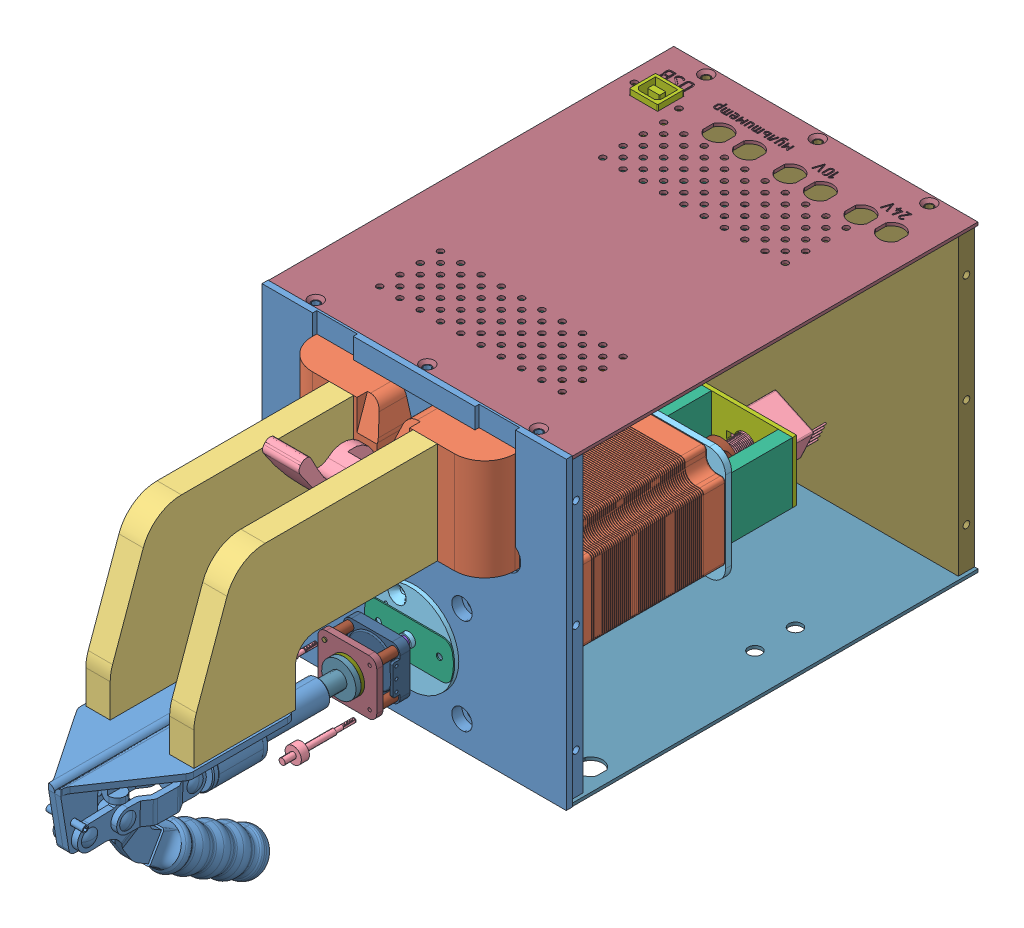
SolidWorks assembly Сборка лнейность, configuration По умолчанию. Lengths in mm.
Overall size (150 180.34 380.2).
57 component instances, 46 part files, 135 mates.
Components (placement in the parent):
- стол-1: стол [По умолчанию] at origin size (150 150 10)
- Nema 23-1: Nema 23 [По умолчанию] at (75 37 -115.5) x (0 -1 0) z (-1 0 0) size (56.72 113.5 73.51)
- подшипник-1: подшипник [По умолчанию] at (75 37 2) x (0.986309 0.164906 0) z (0 0 1) size (26 26 8)
- энкодер-1: энкодер [По умолчанию] at (63.0368 33.7853 -173.6) x (0.90717 -0.420764 0) z (0 0 1) size (21.2 15.9 49.6)
- крышка верхняя-1: крышка верхняя [По умолчанию] at (75 37 8) x (0.789196 -0.614141 0) z (0 0 1) size (44 44 6.7)
- изолятор-1: изолятор [По умолчанию] at (75 37 12) x (0.999997 -0.002629 0) z (0 0 1) size (44 19 0.6)
- ось корпус-1: ось корпус [По умолчанию] at (75 37 2) x (0.996574 0.082709 0) z (0 0 1) size (17.99 18 33.7)
- ось-1: ось [По умолчанию] at (75 37 9.6209) x (0.996574 0.082709 0) z (0 0 1) size (6.5 6.5 30.4)
- стопор оси-1: стопор оси [По умолчанию] at (75.3391 32.914 6.6209) x (-0.98067 -0.081389 0.177938) z (-0.082709 0.996574 0) size (2 2 8.5)
- стойка-1: стойка [По умолчанию] at (55.43 9 -38) x (0 1 0) z (0 0 1) size (56 8 38)
- стойка-2: стойка [По умолчанию] at (102.57 9 -38) x (0 1 0) z (0 0 1) size (56 8 38)
- муфта-1: муфта [По умолчанию] at (75 37 -121.5) x (-0.99255 0.121836 0) z (0 0 -1) size (17.99 18 20)
- основание-1: основание [По умолчанию] at (1.7 1.7 -193) size (146.6 146.6 8)
- стенка бок-1: стенка бок [По умолчанию] at (149.8 148.3 -193) x (0 -1 0) z (-1 0 0) size (146.6 200 1.5) (hidden)
- стенка зад-1: стенка зад [По умолчанию] at (0 149.8 -193) x (1 0 0) z (0 -1 0) size (150 200 1.5)
- стенка перед-1: стенка перед [По умолчанию] at (150 0.2 -193) x (-1 0 0) z (0 1 0) size (150 200 1.5)
- драйвер-1: драйвер [По умолчанию] at (1.7 126.8 -145) x (1 0 0) z (0 -1 0) size (75 118 32)
- стенка бок 2-1: стенка бок 2 [По умолчанию] at (0.2 1.7 -193) x (0 1 0) z (1 0 0) size (146.6 200 1.5)
- стойка для платы-1: стойка для платы [По умолчанию] at (9.7 26.7 -148) x (0 0 1) z (-1 0 0) size (8 8 8)
- стойка для платы-2: стойка для платы [По умолчанию] at (9.7 80.7 -148) x (0 0 1) z (-1 0 0) size (8 8 8)
- стойка для платы-3: стойка для платы [По умолчанию] at (9.7 80.7 -64) x (0 0 1) z (-1 0 0) size (8 8 8)
- стойка для платы-4: стойка для платы [По умолчанию] at (9.7 26.7 -64) x (0 0 1) z (-1 0 0) size (8 8 8)
- плата-1: плата [По умолчанию] at (9.7 18.7 -156) x (0 1 0) z (1 0 0) size (70 100 9)
- прижим-1: прижим [По умолчанию] at (75.5899 43.7042 131.1718) x (0 0 1) z (0 -1 0) size (129.93 55.6 84)
- стойка прижима основа-1: стойка прижима основа [По умолчанию] at (25 140 8) x (0 -1 0) z (0 0 1) size (50 100 17.2)
- стойка прижима держатель-1: стойка прижима держатель [По умолчанию] at (48.35 61.4042 95.2) x (0 1 0) z (1 0 0) size (78.62 120 12)
- стойка прижима держатель-2: стойка прижима держатель [По умолчанию] at (89.65 61.4042 95.2) x (0 1 0) z (1 0 0) size (78.62 120 12)
- плата для замеров-1: плата для замеров [По умолчанию] at (75 37 10) size (150 90 3) (hidden)
- винт-1: винт [По умолчанию] at (86.8379 27.7879 51.4405) x (0.711974 0.702205 0) z (0 0 1) size (8 8 35.5)
- винт-2: винт [По умолчанию] at (63.1621 46.2121 46.6645) x (-0.879742 0.475451 0) z (0 0 1) size (8 8 35.5)
- держатель энкодера пластина-1: держатель энкодера пластина [По умолчанию] at (47 65 -118.5) x (0 -1 0) z (0 0 1) size (56 56 3)
- держатель энкодера стойка-1: держатель энкодера стойка [По умолчанию] at (51.5 52 -118.5) x (0 -1 0) z (1 0 0) size (30 34.6 7)
- держатель энкодера стойка-2: держатель энкодера стойка [По умолчанию] at (91.5 52 -118.5) x (0 -1 0) z (1 0 0) size (30 34.6 7)
- держатель энкодера крышка-1: держатель энкодера крышка [По умолчанию] at (98.5 22 -153.1) x (-1 0 0) z (0 0 -1) size (47 30 2)
- гайка-1: гайка [По умолчанию] at (75 115 -1.7) x (-1 0 0) z (0 0 1) size (13 13 5.9)
- фиксатор-1: фиксатор [По умолчанию] at (60 107.5 -3.2) size (30 15 3)
- п_крышка.stp-2: п_крышка.stp [По умолчанию] at (75 37.0042 34.5225) x (-1 0 0) z (0 0 -1) size (28 26 8.5)
- стойка крышка-1: стойка крышка [По умолчанию] at (86 27.5042 30.9225) size (4.4 4.4 9)
- стойка крышка-2: стойка крышка [По умолчанию] at (64 46.5042 30.9225) size (4.4 4.4 9)
- стойка крышка-3: стойка крышка [По умолчанию] at (64 27.5042 30.9225) size (4.4 4.4 9)
- стойка крышка-4: стойка крышка [По умолчанию] at (86 46.5042 30.9225) size (4.4 4.4 9)
- винт 2-1: винт 2 [По умолчанию] at (64 46.5042 26.1225) size (3.7 3.7 17.3)
- прижим крышки-1: прижим крышки [По умолчанию] at (60.5 23.5042 39.9225) size (29 27 3)
- винт опора крышки-1: винт опора крышки [По умолчанию] at (75 37.0042 47.1225) x (-0.478283 -0.878206 0) z (0 0 -1) size (17 17 37.2)
- шайба прижима-1: шайба прижима [По умолчанию] at (75 37.0042 39.9225) x (-0.50555 -0.862797 0) z (0 0 -1) size (17 17 2)
- резина-1: резина [По умолчанию] at (75 37.0042 42.9225) size (17 17 1.7)
- п_корпус.stp-1: п_корпус.stp [По умолчанию] at (75 37 25.1) x (0.051325 0.998682 0) z (0 0 -1) size (28 36 12.5) (hidden)
- держатель датчика-1: держатель датчика [По умолчанию] at (48.57 66.5 -36.15) x (1 0 0) z (0 -1 0) size (55 25 1.5)
- датчик-1: датчик [По умолчанию] at (81.195 58.34 -3.05) x (0 0 -1) z (0 1 0) size (33.3 10.25 18.74)
- диск датчика-1: диск датчика [По умолчанию] at (75 37 -25) x (-0.996574 -0.082709 0) z (0 0 1) size (37 37 1.5)
- датчик стойка-1: датчик стойка [По умолчанию] at (76.07 60 -33.15) x (1 0 0) z (0 1 0) size (6 6 5)
- датчик стойка-2: датчик стойка [По умолчанию] at (76.07 60 -14.15) x (1 0 0) z (0 1 0) size (6 6 5)
- контакт-1: контакт [По умолчанию] at (75 37.0042 29.5225) size (21.8 21.8 0.8)
- эксцентрик-1: эксцентрик [По умолчанию] at (65.95 117.2509 36.0167) x (0 0.661095 0.750303) z (1 0 0) size (59.77 22.47 18)
- штифт эксцентрика-1: штифт эксцентрика [По умолчанию] at (83.95 115 38) x (0 0.994131 -0.108185) z (-1 0 0) size (6 6 18)
- винт эксцентрика-1: винт эксцентрика [По умолчанию] at (75 115 -23) x (0 1 0) z (0 0 1) size (14 8 68)
- разъем USB-1: разъем USB [По умолчанию] at (7.8 148.3 -176.75) x (1 0 0) z (0 -1 0) size (28 18 18.8)
Mates (geometry in assembly coordinates):
- Параллельность1: parallel anti-aligned: plane of стол-1 through (0 0 0) normal (0 0 -1); plane of Nema 23-1 through (75 37 -36.5) normal (0 0 1)
- Параллельность2: parallel aligned: plane of стол-1 through (0 0 10) normal (0 -1 0); plane of Nema 23-1 through (58 8.85 -38) normal (0 -1 0)
- Концентричный15: concentric anti-aligned: cylinder of Nema 23-1 through (75 37 -130.5) axis (0 0 1) radius 4; cylinder of энкодер-1 through (75 37 -132.5) axis (0 0 -1) radius 3.15
- Совпадение18: coincident anti-aligned: plane of стол-1 through (75 37 2) normal (0 0 1); plane of подшипник-1 through (75 37 2) normal (0 0 -1)
- Концентричный16: concentric anti-aligned: cylinder of стол-1 through (75 37 2) axis (0 0 1) radius 13; cylinder of подшипник-1 through (75 37 10) axis (0 0 -1) radius 13
- Совпадение19: coincident anti-aligned: plane of стол-1 through (75 37 8) normal (0 0 1); plane of крышка верхняя-1 through (75 37 8) normal (0 0 -1)
- Совпадение20: coincident anti-aligned: plane of крышка верхняя-1 through (75 37 12) normal (0 0 1); plane of изолятор-1 through (75 37 12) normal (0 0 -1)
- Концентричный20: concentric anti-aligned: cylinder of крышка верхняя-1 through (75 37 14.7) axis (0 0 -1) radius 3.25; cylinder of изолятор-1 through (75 37 12) axis (0 0 1) radius 3.25
- Концентричный21: concentric anti-aligned: cylinder of подшипник-1 through (75 37 10) axis (0 0 -1) radius 4.5; cylinder of крышка верхняя-1 through (75 37 8) axis (0 0 1) radius 2.5
- Концентричный23: concentric aligned: cylinder of подшипник-1 through (75 37 10) axis (0 0 -1) radius 4.5; cylinder of ось корпус-1 through (75 37 9.7) axis (0 0 -1) radius 4.5
- Концентричный24: concentric anti-aligned: cylinder of ось-1 through (75.2688 33.7611 6.6209) axis (-0.082709 0.996574 0) radius 1; cylinder of стопор оси-1 through (74.6361 41.3849 6.6209) axis (0.082709 -0.996574 0) radius 1
- Расстояние3: distance = 4.1 mm: cylinder of ось-1 through (75 37 -5.3791) axis (0 0 1) radius 3.25; plane of стопор оси-1 through (75.3391 32.914 6.6209) normal (0.082709 -0.996574 0)
- Концентричный25: concentric aligned: cylinder of ось корпус-1 through (75 37 -16.3) axis (0 0 1) radius 3.25; cylinder of ось-1 through (75 37 -5.3791) axis (0 0 1) radius 3.25
- Параллельность3: parallel anti-aligned: cylinder of ось корпус-1 through (75.579 30.024 3) axis (-0.082709 0.996574 0) radius 1; cylinder of стопор оси-1 through (74.6361 41.3849 6.6209) axis (0.082709 -0.996574 0) radius 1
- Совпадение24: coincident anti-aligned: plane of подшипник-1 through (75 37 2) normal (0 0 -1); plane of ось корпус-1 through (75 37 2) normal (0 0 1)
- Совпадение32: coincident anti-aligned: plane of стол-1 through (0 0 0) normal (0 0 -1); plane of стойка-2 through (102.57 9 0) normal (0 0 1)
- Совпадение33: coincident anti-aligned: plane of стол-1 through (0 0 0) normal (0 0 -1); plane of стойка-1 through (55.43 9 0) normal (0 0 1)
- Концентричный29: concentric aligned: cylinder of стол-1 through (98.57 60.57 0) axis (0 0 1) radius 2.5; cylinder of стойка-2 through (98.57 60.57 -38) axis (0 0 1) radius 2.1
- Концентричный30: concentric aligned: cylinder of стол-1 through (98.57 13.43 0) axis (0 0 1) radius 2.5; cylinder of стойка-2 through (98.57 13.43 -38) axis (0 0 1) radius 2.1
- Концентричный31: concentric aligned: cylinder of стол-1 through (51.43 60.57 0) axis (0 0 1) radius 2.5; cylinder of стойка-1 through (51.43 60.57 -38) axis (0 0 1) radius 2.1
- Концентричный32: concentric aligned: cylinder of стол-1 through (51.43 13.43 0) axis (0 0 1) radius 2.5; cylinder of стойка-1 through (51.43 13.43 -38) axis (0 0 1) radius 2.1
- Совпадение34: coincident anti-aligned: plane of Nema 23-1 through (101.15 20 -38) normal (0 0 1); plane of стойка-1 through (55.43 9 -38) normal (0 0 -1)
- Концентричный33: concentric aligned: cylinder of Nema 23-1 through (75 37 -17) axis (0 0 -1) radius 4; cylinder of ось корпус-1 through (75 37 -16) axis (0 0 -1) radius 4
- Концентричный35: concentric aligned: cylinder of Nema 23-1 through (75 37 -130.5) axis (0 0 1) radius 4; cylinder of муфта-1 through (75 37 -131.5) axis (0 0 1) radius 4
- Расстояние4: distance = 1 mm anti-aligned: plane of Nema 23-1 through (75 37 -130.5) normal (0 0 -1); plane of муфта-1 through (75 37 -131.5) normal (0 0 1)
- Расстояние5: distance = 1 mm aligned: plane of энкодер-1 through (75 37 -132.5) normal (0 0 1); plane of муфта-1 through (75 37 -131.5) normal (0 0 1)
- Совпадение40: coincident anti-aligned: plane of основание-1 through (148.3 1.7 -185) normal (1 0 0); plane of стенка бок-1 through (148.3 148.3 -193) normal (-1 0 0)
- Концентричный40: concentric aligned: cylinder of основание-1 through (148.3 128.3 -189) axis (-1 0 0) radius 1.65; cylinder of стенка бок-1 through (149.8 128.3 -189) axis (-1 0 0) radius 2
- Концентричный41: concentric aligned: cylinder of основание-1 through (148.3 21.7 -189) axis (-1 0 0) radius 1.65; cylinder of стенка бок-1 through (149.8 21.7 -189) axis (-1 0 0) radius 2
- Совпадение41: coincident anti-aligned: plane of основание-1 through (1.7 148.3 -185) normal (0 1 0); plane of стенка зад-1 through (0 148.3 -193) normal (0 -1 0)
- Концентричный42: concentric aligned: cylinder of основание-1 through (130 148.3 -189) axis (0 -1 0) radius 1.65; cylinder of стенка зад-1 through (130 149.8 -189) axis (0 -1 0) radius 2
- Концентричный43: concentric anti-aligned: cylinder of стол-1 through (20 133.3 3.5) axis (0 1 0) radius 1.65; cylinder of стенка зад-1 through (20 149.8 3.5) axis (0 -1 0) radius 2
- Совпадение42: coincident anti-aligned: plane of стол-1 through (148.3 1.7 7) normal (0 -1 0); plane of стенка перед-1 through (150 1.7 -193) normal (0 1 0)
- Концентричный45: concentric anti-aligned: cylinder of основание-1 through (20 148.3 -189) axis (0 -1 0) radius 1.65; cylinder of стенка перед-1 through (20 0.2 -189) axis (0 1 0) radius 2
- Концентричный46: concentric anti-aligned: cylinder of основание-1 through (130 148.3 -189) axis (0 -1 0) radius 1.65; cylinder of стенка перед-1 through (130 0.2 -189) axis (0 1 0) radius 2
- Совпадение45: coincident anti-aligned: plane of стол-1 through (1.7 148.3 7) normal (-1 0 0); plane of стенка бок 2-1 through (1.7 1.7 -193) normal (1 0 0)
- Концентричный48: concentric anti-aligned: cylinder of стол-1 through (16.7 21.7 3.5) axis (-1 0 0) radius 1.65; cylinder of стенка бок 2-1 through (0.2 21.7 3.5) axis (1 0 0) radius 2
- Концентричный49: concentric anti-aligned: cylinder of стол-1 through (16.7 128.3 3.5) axis (-1 0 0) radius 1.65; cylinder of стенка бок 2-1 through (0.2 128.3 3.5) axis (1 0 0) radius 2
- Параллельность5: parallel anti-aligned: plane of стенка зад-1 through (0 148.3 -193) normal (0 -1 0); plane of драйвер-1 through (1.7 140.8 -145) normal (0 1 0)
- Совпадение48: coincident anti-aligned: plane of стол-1 through (148.3 148.3 7) normal (1 0 0); plane of стенка бок-1 through (148.3 148.3 -193) normal (-1 0 0)
- Концентричный51: concentric anti-aligned: cylinder of стол-1 through (133.3 21.7 3.5) axis (1 0 0) radius 1.65; cylinder of стенка бок-1 through (149.8 21.7 3.5) axis (-1 0 0) radius 2
- Совпадение49: coincident anti-aligned: plane of стенка бок 2-1 through (1.7 1.7 -193) normal (1 0 0); plane of стойка для платы-4 through (1.7 26.7 -64) normal (-1 0 0)
- Совпадение50: coincident anti-aligned: plane of стенка бок 2-1 through (1.7 1.7 -193) normal (1 0 0); plane of стойка для платы-2 through (1.7 80.7 -148) normal (-1 0 0)
- Совпадение51: coincident anti-aligned: plane of стенка бок 2-1 through (1.7 1.7 -193) normal (1 0 0); plane of стойка для платы-3 through (1.7 80.7 -64) normal (-1 0 0)
- Совпадение52: coincident anti-aligned: plane of стенка бок 2-1 through (1.7 1.7 -193) normal (1 0 0); plane of стойка для платы-1 through (1.7 26.7 -148) normal (-1 0 0)
- Совпадение53: coincident anti-aligned: plane of стойка для платы-3 through (9.7 80.7 -64) normal (1 0 0); plane of плата-1 through (9.7 18.7 -156) normal (-1 0 0)
- Концентричный52: concentric aligned: cylinder of стойка для платы-3 through (1.7 80.7 -64) axis (1 0 0) radius 2; cylinder of плата-1 through (9.7 80.7 -64) axis (1 0 0) radius 2
- Концентричный53: concentric aligned: cylinder of стойка для платы-2 through (1.7 80.7 -148) axis (1 0 0) radius 2; cylinder of плата-1 through (9.7 80.7 -148) axis (1 0 0) radius 2
- Концентричный54: concentric aligned: cylinder of стойка для платы-1 through (1.7 26.7 -148) axis (1 0 0) radius 2; cylinder of плата-1 through (9.7 26.7 -148) axis (1 0 0) radius 2
- Концентричный55: concentric aligned: cylinder of стойка для платы-4 through (1.7 26.7 -64) axis (1 0 0) radius 2; cylinder of плата-1 through (9.7 26.7 -64) axis (1 0 0) radius 2
- Концентричный56: concentric aligned: cylinder of стенка бок 2-1 through (0.2 80.7 -64) axis (1 0 0) radius 2; cylinder of стойка для платы-3 through (1.7 80.7 -64) axis (1 0 0) radius 2
- Концентричный57: concentric aligned: cylinder of стенка бок 2-1 through (0.2 26.7 -64) axis (1 0 0) radius 2; cylinder of стойка для платы-4 through (1.7 26.7 -64) axis (1 0 0) radius 2
- Совпадение74: coincident anti-aligned: plane of драйвер-1 through (1.7 108.8 -145) normal (-1 0 0); plane of стенка бок 2-1 through (1.7 1.7 -193) normal (1 0 0)
- Концентричный61: concentric anti-aligned: cylinder of драйвер-1 through (76.7 118.3 -148) axis (-1 0 0) radius 2.5; cylinder of стенка бок 2-1 through (0.2 118.3 -148) axis (1 0 0) radius 2
- Концентричный69: concentric aligned: cylinder of стол-1 through (75 115 0) axis (0 0 1) radius 3; cylinder of стойка прижима основа-1 through (75 115 8) axis (0 0 1) radius 3
- Совпадение81: coincident anti-aligned: plane of стол-1 through (25 90 8) normal (0 1 0); plane of стойка прижима основа-1 through (25 90 25.2) normal (0 -1 0)
- Совпадение82: coincident anti-aligned: plane of стойка прижима основа-1 through (25 140 25.2) normal (0 0 1); plane of стойка прижима держатель-1 through (-46.0026 90 25.2) normal (0 0 -1)
- Совпадение83: coincident anti-aligned: plane of стойка прижима основа-1 through (25 140 25.2) normal (0 0 1); plane of стойка прижима держатель-2 through (-4.7026 90 25.2) normal (0 0 -1)
- Концентричный70: concentric aligned: cylinder of стойка прижима основа-1 through (95.65 100 25.2) axis (0 0 -1) radius 3; cylinder of стойка прижима держатель-2 through (95.65 100 55.2) axis (0 0 -1) radius 2.5
- Параллельность10: parallel aligned: plane of стол-1 through (0 150 10) normal (0 1 0); plane of прижим-1 through (52.2 61.4042 146.67) normal (0 1 0)
- Концентричный78: concentric aligned: cylinder of стойка прижима основа-1 through (54.35 130 25.2) axis (0 0 -1) radius 3; cylinder of стойка прижима держатель-1 through (54.35 130 55.2) axis (0 0 -1) radius 2.5
- Концентричный79: concentric aligned: cylinder of прижим-1 through (95.65 63.1042 136.2) axis (0 -1 0) radius 2.6; cylinder of стойка прижима держатель-2 through (95.65 81.4042 136.2) axis (0 -1 0) radius 2.5
- Совпадение87: coincident anti-aligned: plane of прижим-1 through (97.8 61.4042 146.67) normal (0 1 0); plane of стойка прижима держатель-2 through (101.65 61.4042 95.2) normal (0 -1 0)
- Концентричный80: concentric aligned: cylinder of крышка верхняя-1 through (75 37 12) axis (0 0 -1) radius 22; cylinder of плата для замеров-1 through (75 37 13) axis (0 0 -1) radius 22
- Концентричный81: concentric anti-aligned: cylinder of крышка верхняя-1 through (86.8379 27.7879 8) axis (0 0 1) radius 0.8; cylinder of винт-1 through (86.8379 27.7879 61.4405) axis (0 0 -1) radius 1
- Концентричный82: concentric anti-aligned: cylinder of крышка верхняя-1 through (63.1621 46.2121 8) axis (0 0 1) radius 0.8; cylinder of винт-2 through (63.1621 46.2121 56.6645) axis (0 0 -1) radius 1
- Совпадение92: coincident anti-aligned: plane of Nema 23-1 through (75 37 -115.5) normal (0 0 -1); plane of держатель энкодера пластина-1 through (95 17 -115.5) normal (0 0 1)
- Концентричный84: concentric anti-aligned: cylinder of Nema 23-1 through (59 11.67 -111.5) axis (0 0 -1) radius 1.25; cylinder of держатель энкодера пластина-1 through (59 11.67 -118.5) axis (0 0 1) radius 1.5
- Концентричный85: concentric anti-aligned: cylinder of Nema 23-1 through (91 62.33 -111.5) axis (0 0 -1) radius 1.25; cylinder of держатель энкодера пластина-1 through (91 62.33 -118.5) axis (0 0 1) radius 1.5
- Совпадение93: coincident anti-aligned: plane of держатель энкодера пластина-1 through (95 17 -118.5) normal (0 0 -1); plane of держатель энкодера стойка-1 through (58.5 52 -118.5) normal (0 0 1)
- Совпадение94: coincident anti-aligned: plane of держатель энкодера пластина-1 through (95 17 -118.5) normal (0 0 -1); plane of держатель энкодера стойка-2 through (98.5 52 -118.5) normal (0 0 1)
- Совпадение95: coincident anti-aligned: plane of держатель энкодера стойка-1 through (58.5 52 -153.1) normal (0 0 -1); plane of держатель энкодера крышка-1 through (98.5 22 -153.1) normal (0 0 1)
- Концентричный94: concentric aligned: cylinder of держатель энкодера стойка-2 through (95 48 -118.5) axis (0 0 -1) radius 1.25; cylinder of держатель энкодера крышка-1 through (95 48 -153.1) axis (0 0 -1) radius 1.5
- Концентричный95: concentric anti-aligned: cylinder of держатель энкодера пластина-1 through (55 26 -118.5) axis (0 0 1) radius 1.5; cylinder of держатель энкодера стойка-1 through (55 26 -118.5) axis (0 0 -1) radius 1.25
- Концентричный97: concentric anti-aligned: cylinder of держатель энкодера пластина-1 through (55 48 -118.5) axis (0 0 1) radius 1.5; cylinder of держатель энкодера стойка-1 through (55 48 -118.5) axis (0 0 -1) radius 1.25
- Концентричный98: concentric anti-aligned: cylinder of держатель энкодера пластина-1 through (95 26 -118.5) axis (0 0 1) radius 1.5; cylinder of держатель энкодера стойка-2 through (95 26 -118.5) axis (0 0 -1) radius 1.25
- Концентричный99: concentric anti-aligned: cylinder of держатель энкодера пластина-1 through (95 48 -118.5) axis (0 0 1) radius 1.5; cylinder of держатель энкодера стойка-2 through (95 48 -118.5) axis (0 0 -1) radius 1.25
- Концентричный100: concentric aligned: cylinder of держатель энкодера стойка-1 through (55 26 -118.5) axis (0 0 -1) radius 1.25; cylinder of держатель энкодера крышка-1 through (55 26 -153.1) axis (0 0 -1) radius 1.5
- Совпадение96: coincident anti-aligned: plane of стол-1 through (0 0 0) normal (0 0 -1); plane of гайка-1 through (75 115 0) normal (0 0 1)
- Совпадение97: coincident anti-aligned: plane of стол-1 through (69.2265 115 4) normal (0.866025 -0.5 0); plane of гайка-1 through (72.1132 120 25.3753) normal (-0.866025 0.5 0)
- Концентричный102: concentric aligned: cylinder of стол-1 through (75 115 0) axis (0 0 1) radius 3; cylinder of гайка-1 through (75 115 -1.7) axis (0 0 1) radius 2.5
- Совпадение98: coincident aligned: circle of гайка-1; plane of фиксатор-1 through (75 115 -1.7) normal (0 0 1)
- Концентричный103: concentric aligned: cylinder of стол-1 through (75 115 0) axis (0 0 1) radius 3; cylinder of фиксатор-1 through (75 115 -3.2) axis (0 0 1) radius 3.25
- Совпадение99: coincident anti-aligned: plane of стол-1 through (0 0 10) normal (0 0 1); plane of плата для замеров-1 through (149 89 10) normal (0 0 -1)
- Параллельность12: parallel aligned: plane of стол-1 through (1.7 148.3 7) normal (-1 0 0); plane of плата для замеров-1 through (0 89 13) normal (-1 0 0)
- Совпадение100: coincident aligned: plane of стойка крышка-3 through (64 27.5042 30.9225) normal (0 0 -1); plane of стойка крышка-4 through (86 46.5042 30.9225) normal (0 0 -1)
- Совпадение101: coincident aligned: plane of стойка крышка-2 through (64 46.5042 30.9225) normal (0 0 -1); plane of стойка крышка-3 through (64 27.5042 30.9225) normal (0 0 -1)
- Совпадение102: coincident aligned: plane of стойка крышка-1 through (86 27.5042 30.9225) normal (0 0 -1); plane of стойка крышка-2 through (64 46.5042 30.9225) normal (0 0 -1)
- Совпадение103: coincident anti-aligned: plane of п_крышка.stp-2 through (75 37.0042 30.9225) normal (0 0 1); plane of стойка крышка-1 through (86 27.5042 30.9225) normal (0 0 -1)
- Концентричный104: concentric anti-aligned: cylinder of п_крышка.stp-2 through (86 27.5042 -2.0775) axis (0 0 1) radius 1.2; cylinder of стойка крышка-1 through (86 27.5042 39.9225) axis (0 0 -1) radius 1.2
- Концентричный105: concentric anti-aligned: cylinder of п_крышка.stp-2 through (86 46.5042 -2.0775) axis (0 0 1) radius 1.2; cylinder of стойка крышка-4 through (86 46.5042 39.9225) axis (0 0 -1) radius 1.2
- Концентричный106: concentric anti-aligned: cylinder of п_крышка.stp-2 through (64 46.5042 -2.0775) axis (0 0 1) radius 1.2; cylinder of стойка крышка-2 through (64 46.5042 39.9225) axis (0 0 -1) radius 1.2
- Концентричный107: concentric anti-aligned: cylinder of п_крышка.stp-2 through (64 27.5042 -2.0775) axis (0 0 1) radius 1.2; cylinder of стойка крышка-3 through (64 27.5042 39.9225) axis (0 0 -1) radius 1.2
- Концентричный108: concentric anti-aligned: cylinder of п_крышка.stp-2 through (64 46.5042 -2.0775) axis (0 0 1) radius 1.2; cylinder of винт 2-1 through (64 46.5042 63.5509) axis (0 0 -1) radius 1
- Совпадение104: coincident anti-aligned: plane of п_крышка.stp-2 through (64 46.5042 27.5225) normal (0 0 -1); plane of винт 2-1 through (64 46.5042 27.5225) normal (0 0 1)
- Совпадение105: coincident anti-aligned: plane of стойка крышка-2 through (64 46.5042 39.9225) normal (0 0 1); plane of прижим крышки-1 through (64.5 27.5042 39.9225) normal (0 0 -1)
- Концентричный109: concentric anti-aligned: cylinder of стойка крышка-4 through (86 46.5042 39.9225) axis (0 0 -1) radius 1.2; cylinder of прижим крышки-1 through (86 46.5042 39.9225) axis (0 0 1) radius 0.8
- Концентричный110: concentric anti-aligned: cylinder of стойка крышка-3 through (64 27.5042 39.9225) axis (0 0 -1) radius 1.2; cylinder of прижим крышки-1 through (64 27.5042 39.9225) axis (0 0 1) radius 0.8
- Концентричный111: concentric aligned: cylinder of прижим-1 through (75 37.0042 132.1147) axis (0 0 -1) radius 6.35; cylinder of винт опора крышки-1 through (75 37.0042 77.1225) axis (0 0 -1) radius 4
- Концентричный112: concentric aligned: cylinder of прижим крышки-1 through (75 37.0042 39.9225) axis (0 0 1) radius 4.5; cylinder of винт опора крышки-1 through (75 37.0042 39.9225) axis (0 0 1) radius 4
- Концентричный113: concentric aligned: cylinder of прижим-1 through (54.35 63.1042 102.2) axis (0 -1 0) radius 2.6; cylinder of стойка прижима держатель-1 through (54.35 81.4042 102.2) axis (0 -1 0) radius 2.5
- Концентричный114: concentric anti-aligned: cylinder of винт опора крышки-1 through (75 37.0042 39.9225) axis (0 0 1) radius 4; circle of шайба прижима-1
- Совпадение108: coincident anti-aligned: plane of винт опора крышки-1 through (75 37.0042 39.9225) normal (0 0 -1); plane of шайба прижима-1 through (75 37.0042 39.9225) normal (0 0 1)
- Совпадение109: coincident anti-aligned: plane of винт опора крышки-1 through (75 37.0042 44.6225) normal (0 0 -1); plane of резина-1 through (75 37.0042 44.6225) normal (0 0 1)
- Концентричный115: concentric anti-aligned: cylinder of винт опора крышки-1 through (75 37.0042 39.9225) axis (0 0 1) radius 4; cylinder of резина-1 through (75 37.0042 44.6225) axis (0 0 -1) radius 4
- Совпадение110: coincident anti-aligned: plane of прижим крышки-1 through (64.5 27.5042 42.9225) normal (0 0 1); plane of резина-1 through (75 37.0042 42.9225) normal (0 0 -1)
- Параллельность13: parallel aligned: plane of стойка прижима основа-1 through (25 90 25.2) normal (0 -1 0); plane of прижим крышки-1 through (64.5 23.5042 42.9225) normal (0 -1 0)
- Совпадение112: coincident anti-aligned: plane of стол-1 through (0 0 8) normal (0 0 1); plane of стойка прижима основа-1 through (25 140 8) normal (0 0 -1)
- Совпадение113: coincident anti-aligned: plane of изолятор-1 through (75 37 12.6) normal (0 0 1); plane of п_корпус.stp-1 through (75 37 12.6) normal (0 0 -1)
- Концентричный116: concentric aligned: cylinder of крышка верхняя-1 through (75 37 14.7) axis (0 0 -1) radius 3.25; cylinder of п_корпус.stp-1 through (75 37 25.1) axis (0 0 -1) radius 2.5
- Совпадение114: coincident anti-aligned: plane of стойка-2 through (102.57 65 0) normal (0 1 0); plane of держатель датчика-1 through (48.57 65 -36.15) normal (0 -1 0)
- Параллельность16: parallel aligned: plane of стойка-1 through (47.43 9 0) normal (-1 0 0); plane of держатель датчика-1 through (48.57 65 -36.15) normal (-1 0 0)
- Концентричный123: concentric anti-aligned: cylinder of Nema 23-1 through (75 37 -17) axis (0 0 -1) radius 4; cylinder of диск датчика-1 through (75 37 -25) axis (0 0 1) radius 4
- Совпадение116: coincident anti-aligned: plane of ось корпус-1 through (75 37 -24) normal (0 0 -1); plane of диск датчика-1 through (75 37 -24) normal (0 0 1)
- Параллельность17: parallel aligned: plane of ось корпус-1 through (42.1379 33.9716 -26) normal (-0.082709 0.996574 0); plane of диск датчика-1 through (72.5324 36.3437 -25) normal (-0.082709 0.996574 0)
- Совпадение118: coincident aligned: plane of датчик стойка-1 through (76.07 65 -33.15) normal (0 1 0); plane of датчик стойка-2 through (76.07 65 -14.15) normal (0 1 0)
- Совпадение119: coincident anti-aligned: plane of держатель датчика-1 through (48.57 65 -36.15) normal (0 -1 0); plane of датчик стойка-2 through (76.07 65 -14.15) normal (0 1 0)
- Концентричный124: concentric aligned: cylinder of держатель датчика-1 through (76.07 66.5 -33.15) axis (0 -1 0) radius 1.6; cylinder of датчик стойка-1 through (76.07 65 -33.15) axis (0 -1 0) radius 1.65
- Концентричный125: concentric aligned: cylinder of держатель датчика-1 through (76.07 66.5 -14.15) axis (0 -1 0) radius 1.6; cylinder of датчик стойка-2 through (76.07 65 -14.15) axis (0 -1 0) radius 1.65
- Совпадение120: coincident anti-aligned: plane of датчик-1 through (81.195 60 -3.05) normal (0 1 0); plane of датчик стойка-2 through (76.07 60 -14.15) normal (0 -1 0)
- Концентричный126: concentric anti-aligned: cylinder of датчик-1 through (76.07 58.34 -14.15) axis (0 1 0) radius 1.7; cylinder of датчик стойка-2 through (76.07 65 -14.15) axis (0 -1 0) radius 1.65
- Концентричный127: concentric anti-aligned: cylinder of датчик-1 through (76.07 58.34 -33.15) axis (0 1 0) radius 1.7; cylinder of датчик стойка-1 through (76.07 65 -33.15) axis (0 -1 0) radius 1.65
- Концентричный128: concentric anti-aligned: cylinder of стойка-2 through (98.57 45 -19) axis (0 1 0) radius 1.25; cylinder of держатель датчика-1 through (98.57 66.5 -19) axis (0 -1 0) radius 1.6
- Совпадение121: coincident anti-aligned: plane of п_крышка.stp-2 through (75 37.0042 30.3225) normal (0 0 -1); plane of контакт-1 through (75 37.0042 30.3225) normal (0 0 1)
- Концентричный129: concentric aligned: cylinder of п_крышка.stp-2 through (75 37.0042 30.2225) axis (0 0 -1) radius 3.5; cylinder of контакт-1 through (75 37.0042 30.3225) axis (0 0 -1) radius 4.9
- Концентричный130: concentric anti-aligned: cylinder of стол-1 through (75 115 0) axis (0 0 1) radius 3; cylinder of винт эксцентрика-1 through (75 115 32) axis (0 0 -1) radius 3
- Параллельность18: parallel anti-aligned: plane of стойка прижима держатель-1 through (60.35 61.4042 95.2) normal (1 0 0); plane of винт эксцентрика-1 through (71 115 38) normal (-1 0 0)
- Концентричный131: concentric anti-aligned: cylinder of эксцентрик-1 through (70.5147 115 38) axis (1 0 0) radius 3; cylinder of винт эксцентрика-1 through (79 115 38) axis (-1 0 0) radius 3
- Совпадение123: coincident anti-aligned: plane of эксцентрик-1 through (79 118.2322 20.4913) normal (-1 0 0); plane of винт эксцентрика-1 through (79 115 38) normal (1 0 0)
- Концентричный132: concentric aligned: cylinder of эксцентрик-1 through (65.95 115 38) axis (1 0 0) radius 2.1; cylinder of штифт эксцентрика-1 through (70.95 115 38) axis (1 0 0) radius 3
- Совпадение124: coincident aligned: plane of эксцентрик-1 through (83.95 117.2509 36.0167) normal (1 0 0); plane of штифт эксцентрика-1 through (83.95 115 38) normal (1 0 0)
- Расстояние6: distance = 23 mm aligned: plane of стол-1 through (0 0 0) normal (0 0 -1); plane of винт эксцентрика-1 through (75 115 -23) normal (0 0 -1)
- Совпадение125: coincident anti-aligned: plane of стенка зад-1 through (0 148.3 -193) normal (0 -1 0); plane of разъем USB-1 through (9.3 148.3 -175.25) normal (0 1 0)
- Концентричный133: concentric aligned: cylinder of стенка зад-1 through (27.8 148.3 -167.75) axis (0 1 0) radius 1.55; cylinder of разъем USB-1 through (27.8 133.8 -167.75) axis (0 1 0) radius 1.25
- Концентричный134: concentric aligned: cylinder of стенка зад-1 through (5.8 148.3 -167.75) axis (0 1 0) radius 1.55; cylinder of разъем USB-1 through (5.8 133.8 -167.75) axis (0 1 0) radius 1.25
